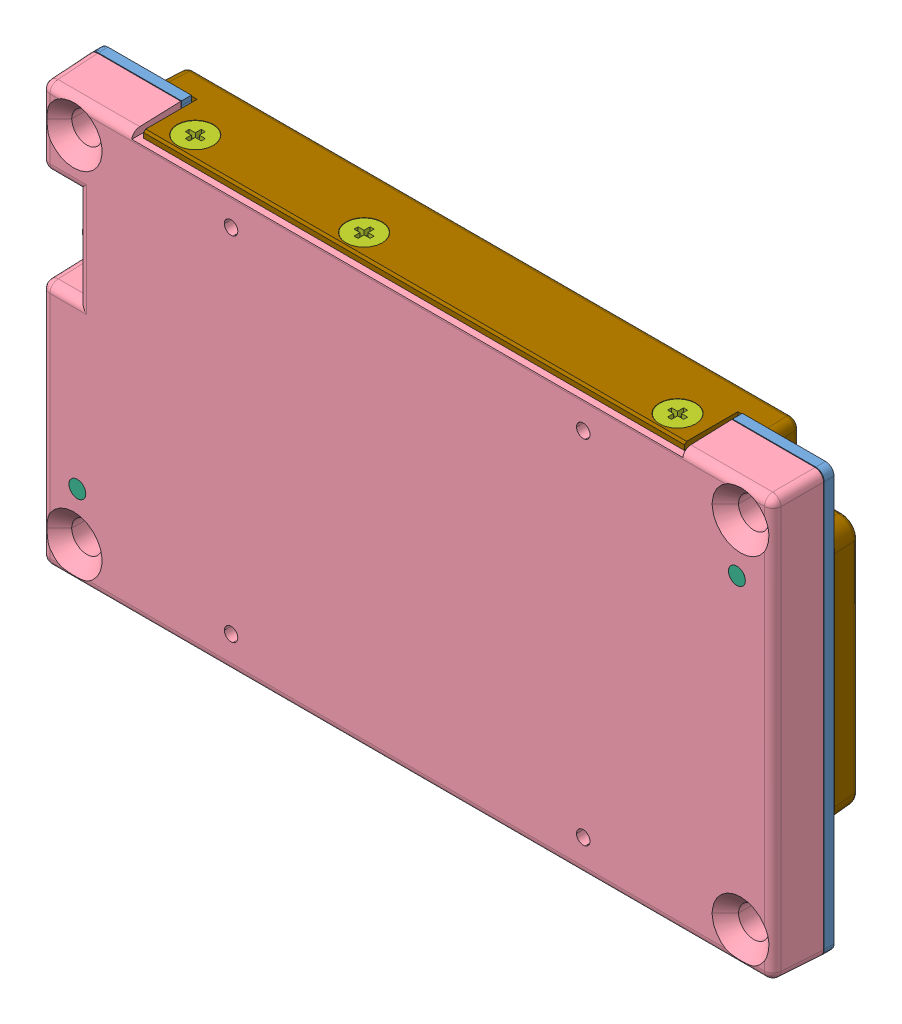
SolidWorks assembly P3310_module, configuration Default. Lengths in mm.
Overall size (87.74 50.06 12.14).
23 component instances, 10 part files, 0 mates.
Components (placement in the parent):
- P3310_module.stp-1: P3310_module.stp [Default] at origin size (87.74 50.06 12.14)
  - 244-83310-1000-C03_ASM.stp-1: 244-83310-1000-C03_ASM.stp [Default] at origin size (87 50 7.77)
    - 142-83310-1000-C03.stp-1: 142-83310-1000-C03.stp [Default] at origin size (87 50 1.16)
    - 080-0550-000_2.stp-1: 080-0550-000_2.stp [Default] at (-2.36 33.789 1.164) size (3.63 4.07 1.47)
    - 080-0550-000_2.stp-2: 080-0550-000_2.stp [Default] at (-2.36 28.232 1.164) size (3.63 4.07 1.47)
    - 080-1337-000_1.stp-1: 080-1337-000_1.stp [Default] at (39.5 3.4 0) x (1 0 0) z (0 0 -1) size (70.15 10.74 5.05)
  - TTP-186-DIE-REFERENCE-C00_ASM.stp-1: TTP-186-DIE-REFERENCE-C00_ASM.stp [Default] at (0.432 5.918 1.244) size (87.03 50.03 8.01)
    - 094-0021-004_1.stp-1: 094-0021-004_1.stp [Default] at origin size (87.03 50.03 5.85)
    - 153-0369-000-PRELOAD.stp-1: 153-0369-000-PRELOAD.stp [Default] at (26.3174 29.151 5) x (1 0 0) z (0 1 0) size (8.11 3.29 7.91)
    - 153-0369-000-PRELOAD.stp-2: 153-0369-000-PRELOAD.stp [Default] at (51.8674 29.151 5) x (1 0 0) z (0 1 0) size (8.11 3.29 7.91)
    - 153-0369-000-PRELOAD.stp-3: 153-0369-000-PRELOAD.stp [Default] at (39.0874 5.9953 5) x (1 0 0) z (0 1 0) size (8.11 3.29 7.91)
    - PIN_8_00-DIE-REFERENCE-P3310.stp-1: PIN_8_00-DIE-REFERENCE-P3310.stp [Default] at (0 0 -1.2) x (-1 0 0) z (0 1 0) size (2 8 2)
    - PIN_8_00-DIE-REFERENCE-P3310.stp-2: PIN_8_00-DIE-REFERENCE-P3310.stp [Default] at (78.138 30.162 -1.2) x (-1 0 0) z (0 1 0) size (2 8 2)
    - 153-0368-000.stp-1: 153-0368-000.stp [Default] at (39.0874 5.9953 1.73) x (-1 0 0) z (0 1 0) size (4.25 3.7 4.25)
    - 153-0368-000.stp-2: 153-0368-000.stp [Default] at (26.3174 29.151 1.73) x (-1 0 0) z (0 1 0) size (4.25 3.7 4.25)
    - 153-0368-000.stp-3: 153-0368-000.stp [Default] at (51.8674 29.151 1.73) x (-1 0 0) z (0 1 0) size (4.25 3.7 4.25)
    - PRESSURE-PLATE-P3310-C01.stp-1: PRESSURE-PLATE-P3310-C01.stp [Default] at (39.0874 18.8953 2.9656) x (-1 0 0) z (0 -1 0) size (30.37 2.6 29.12)
  - P3310-BOTTOM-COVER--CNC-0316.stp-1: P3310-BOTTOM-COVER--CNC-0316.stp [Default] at (83 8.88 -0.1484) x (-1 0 0) z (0 -1 0) size (87.47 9.23 36.87)
  - 155-0343-000.stp-1: 155-0343-000.stp [Default] at (79 21 -1.1784) x (-1 0 0) z (0 0 -1) size (5.55 5.55 7.54)
  - 155-0343-000.stp-2: 155-0343-000.stp [Default] at (0 21 -1.1784) x (-1 0 0) z (0 0 -1) size (5.55 5.55 7.54)
  - 153-0368-000.stp-1: 153-0368-000.stp [Default] at (68.1416 45.009 3.6756) x (-1 0 0) z (0 0 1) size (4.25 3.7 4.25)
  - 153-0368-000.stp-2: 153-0368-000.stp [Default] at (31 45.009 3.6756) x (-1 0 0) z (0 0 1) size (4.25 3.7 4.25)
  - 153-0368-000.stp-3: 153-0368-000.stp [Default] at (11 45.009 3.6756) x (-1 0 0) z (0 0 1) size (4.25 3.7 4.25)
